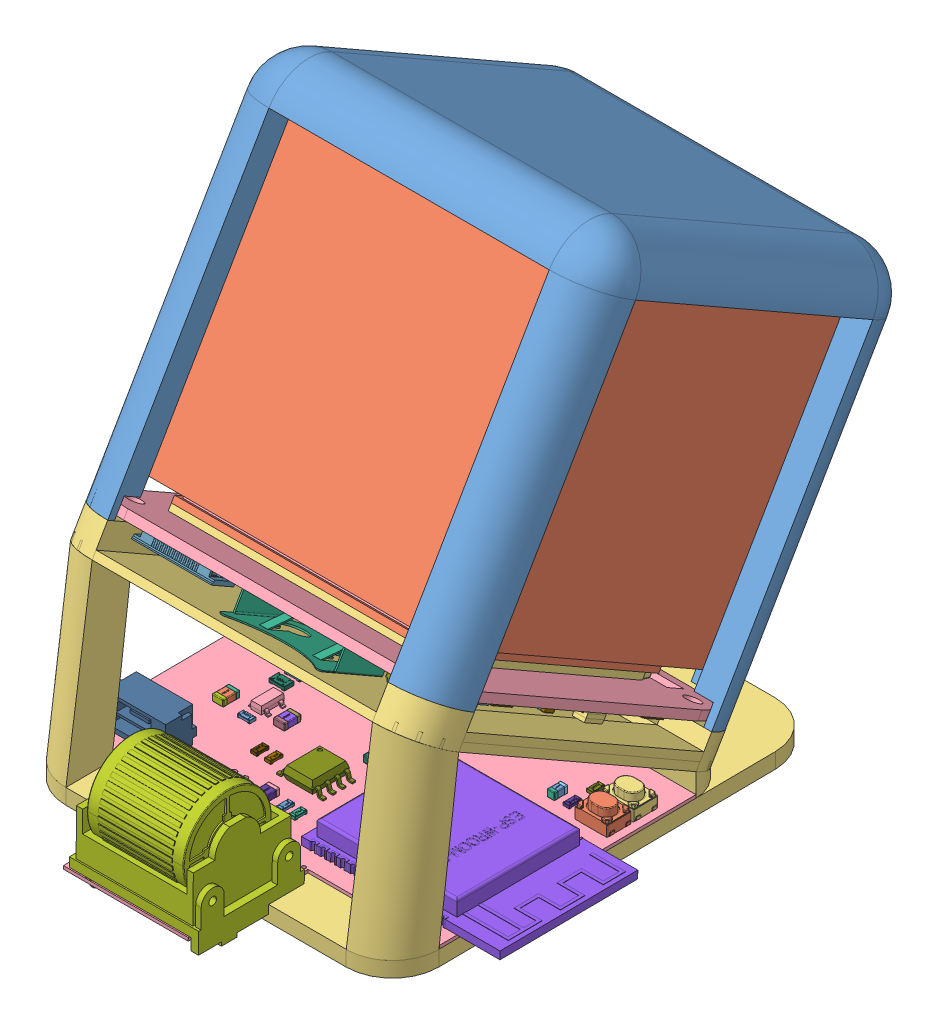
SolidWorks assembly main, configuration 默认. Lengths in mm. (continued)
Components (placement in the parent): (continued)
- PCB_deskclok_ext_2021-02-23-1: PCB_deskclok_ext_2021-02-23 [默认] at (-67.7963 -6.5111 77.6298) x (0.999924 -0.008726 -0.008727) z (0.008727 0.999962 0) size (54.77 48.92 16.75)
  - PCB_deskclok_ext_2021-02-23(2)^PCB_deskclok_ext_2021-02-23-1: PCB_deskclok_ext_2021-02-23(2)^PCB_deskclok_ext_2021-02-23 [默认] at origin size (54.77 48.92 16.75) (virtual)
    - Board^PCB_deskclok_ext_2021-02-23(2)_PCB_deskclok_ext_2021-02-23-1: Board^PCB_deskclok_ext_2021-02-23(2)_PCB_deskclok_ext_2021-02-23 [默认] at origin size (48 48.92 0.41) (virtual)
      - Open CASCADE STEP translator 6.8 2.1.1^Board_PCB_deskclok_ext_2021-02-23(2)_PCB_deskclok_ext_2021-02-23-1: Open CASCADE STEP translator 6.8 2.1.1^Board_PCB_deskclok_ext_2021-02-23(2)_PCB_deskclok_ext_2021-02-23 [默认] at (0 0 -0.4115) size (48 48.92 0.41) (virtual)
        - Open CASCADE STEP translator 6.8 2.1.1.1^Open CASCADE STEP translator 6.8 2.1.1_Board_PCB_deskclok_ext_2021-02-23(2)_PCB_deskclok_ext_2021-02-23-1: Open CASCADE STEP translator 6.8 2.1.1.1^Open CASCADE STEP translator 6.8 2.1.1_Board_PCB_deskclok_ext_2021-02-23(2)_PCB_deskclok_ext_2021-02-23 [默认] at origin size (48 48.92 0.41) (virtual)
    - LED6^PCB_deskclok_ext_2021-02-23(2)_PCB_deskclok_ext_2021-02-23-1: LED6^PCB_deskclok_ext_2021-02-23(2)_PCB_deskclok_ext_2021-02-23 [默认] at origin size (2.13 1.25 1.24) (virtual)
      - everlight-17-21-0805LED-GREEN^LED6_PCB_deskclok_ext_2021-02-23(2)_PCB_deskclok_ext_2021-02-23-1: everlight-17-21-0805LED-GREEN^LED6_PCB_deskclok_ext_2021-02-23(2)_PCB_deskclok_ext_2021-02-23 [默认] at (47.3416 90.4196 0.3048) x (1 0 0) z (0 -1 0) size (2.13 1.24 1.25) (virtual)
    - R9^PCB_deskclok_ext_2021-02-23(2)_PCB_deskclok_ext_2021-02-23-1: R9^PCB_deskclok_ext_2021-02-23(2)_PCB_deskclok_ext_2021-02-23 [默认] at origin size (0.8 1.6 0.42) (virtual)
      - User_Library-Res-0603^R9_PCB_deskclok_ext_2021-02-23(2)_PCB_deskclok_ext_2021-02-23-1: User_Library-Res-0603^R9_PCB_deskclok_ext_2021-02-23(2)_PCB_deskclok_ext_2021-02-23 [默认] at (69.3811 64.135 0) x (0 -1 0) z (-1 0 0) size (1.6 0.42 0.8) (virtual)
    - C6^PCB_deskclok_ext_2021-02-23(2)_PCB_deskclok_ext_2021-02-23-1: C6^PCB_deskclok_ext_2021-02-23(2)_PCB_deskclok_ext_2021-02-23 [默认] at origin size (1.45 2.2 0.88) (virtual)
      - c0805c101k5gactu^C6_PCB_deskclok_ext_2021-02-23(2)_PCB_deskclok_ext_2021-02-23-1: c0805c101k5gactu^C6_PCB_deskclok_ext_2021-02-23(2)_PCB_deskclok_ext_2021-02-23 [默认] at (28.223 186.145 -10.6426) x (0 1 0) z (1 0 0) size (2.2 0.88 1.45) (virtual)
        - Open CASCADE STEP translator 6.8 2.4.1.1^c0805c101k5gactu_C6_PCB_deskclok_ext_2021-02-23(2)_PCB_deskclok_ext_2021-02-23-1: Open CASCADE STEP translator 6.8 2.4.1.1^c0805c101k5gactu_C6_PCB_deskclok_ext_2021-02-23(2)_PCB_deskclok_ext_2021-02-23 [默认] at origin size (2 0.86 1.43) (virtual)
        - Open CASCADE STEP translator 6.8 2.4.1.2^c0805c101k5gactu_C6_PCB_deskclok_ext_2021-02-23(2)_PCB_deskclok_ext_2021-02-23-1: Open CASCADE STEP translator 6.8 2.4.1.2^c0805c101k5gactu_C6_PCB_deskclok_ext_2021-02-23(2)_PCB_deskclok_ext_2021-02-23 [默认] at origin size (0.34 0 0.18) (virtual)
        - Open CASCADE STEP translator 6.8 2.4.1.3^c0805c101k5gactu_C6_PCB_deskclok_ext_2021-02-23(2)_PCB_deskclok_ext_2021-02-23-1: Open CASCADE STEP translator 6.8 2.4.1.3^c0805c101k5gactu_C6_PCB_deskclok_ext_2021-02-23(2)_PCB_deskclok_ext_2021-02-23 [默认] at origin size (0.41 0 0.18) (virtual)
        - Open CASCADE STEP translator 6.8 2.4.1.4^c0805c101k5gactu_C6_PCB_deskclok_ext_2021-02-23(2)_PCB_deskclok_ext_2021-02-23-1: Open CASCADE STEP translator 6.8 2.4.1.4^c0805c101k5gactu_C6_PCB_deskclok_ext_2021-02-23(2)_PCB_deskclok_ext_2021-02-23 [默认] at origin size (0.21 0 0.18) (virtual)
        - Open CASCADE STEP translator 6.8 2.4.1.5^c0805c101k5gactu_C6_PCB_deskclok_ext_2021-02-23(2)_PCB_deskclok_ext_2021-02-23-1: Open CASCADE STEP translator 6.8 2.4.1.5^c0805c101k5gactu_C6_PCB_deskclok_ext_2021-02-23(2)_PCB_deskclok_ext_2021-02-23 [默认] at origin size (0.5 0.88 1.45) (virtual)
        - Open CASCADE STEP translator 6.8 2.4.1.6^c0805c101k5gactu_C6_PCB_deskclok_ext_2021-02-23(2)_PCB_deskclok_ext_2021-02-23-1: Open CASCADE STEP translator 6.8 2.4.1.6^c0805c101k5gactu_C6_PCB_deskclok_ext_2021-02-23(2)_PCB_deskclok_ext_2021-02-23 [默认] at origin size (0.5 0.88 1.45) (virtual)
    - C9^PCB_deskclok_ext_2021-02-23(2)_PCB_deskclok_ext_2021-02-23-1: C9^PCB_deskclok_ext_2021-02-23(2)_PCB_deskclok_ext_2021-02-23 [默认] at origin size (1.45 2.2 0.88) (virtual)
      - c0805c101k5gactu^C9_PCB_deskclok_ext_2021-02-23(2)_PCB_deskclok_ext_2021-02-23-1: c0805c101k5gactu^C9_PCB_deskclok_ext_2021-02-23(2)_PCB_deskclok_ext_2021-02-23 [默认] at (117.778 -11.52 -10.6426) x (0 -1 0) z (-1 0 0) size (2.2 0.88 1.45) (virtual)
        - Open CASCADE STEP translator 6.8 2.4.1.1^c0805c101k5gactu_C9_PCB_deskclok_ext_2021-02-23(2)_PCB_deskclok_ext_2021-02-23-1: Open CASCADE STEP translator 6.8 2.4.1.1^c0805c101k5gactu_C9_PCB_deskclok_ext_2021-02-23(2)_PCB_deskclok_ext_2021-02-23 [默认] at origin size (2 0.86 1.43) (virtual)
        - Open CASCADE STEP translator 6.8 2.4.1.2^c0805c101k5gactu_C9_PCB_deskclok_ext_2021-02-23(2)_PCB_deskclok_ext_2021-02-23-1: Open CASCADE STEP translator 6.8 2.4.1.2^c0805c101k5gactu_C9_PCB_deskclok_ext_2021-02-23(2)_PCB_deskclok_ext_2021-02-23 [默认] at origin size (0.34 0 0.18) (virtual)
        - Open CASCADE STEP translator 6.8 2.4.1.3^c0805c101k5gactu_C9_PCB_deskclok_ext_2021-02-23(2)_PCB_deskclok_ext_2021-02-23-1: Open CASCADE STEP translator 6.8 2.4.1.3^c0805c101k5gactu_C9_PCB_deskclok_ext_2021-02-23(2)_PCB_deskclok_ext_2021-02-23 [默认] at origin size (0.41 0 0.18) (virtual)
        - Open CASCADE STEP translator 6.8 2.4.1.4^c0805c101k5gactu_C9_PCB_deskclok_ext_2021-02-23(2)_PCB_deskclok_ext_2021-02-23-1: Open CASCADE STEP translator 6.8 2.4.1.4^c0805c101k5gactu_C9_PCB_deskclok_ext_2021-02-23(2)_PCB_deskclok_ext_2021-02-23 [默认] at origin size (0.21 0 0.18) (virtual)
        - Open CASCADE STEP translator 6.8 2.4.1.5^c0805c101k5gactu_C9_PCB_deskclok_ext_2021-02-23(2)_PCB_deskclok_ext_2021-02-23-1: Open CASCADE STEP translator 6.8 2.4.1.5^c0805c101k5gactu_C9_PCB_deskclok_ext_2021-02-23(2)_PCB_deskclok_ext_2021-02-23 [默认] at origin size (0.5 0.88 1.45) (virtual)
        - Open CASCADE STEP translator 6.8 2.4.1.6^c0805c101k5gactu_C9_PCB_deskclok_ext_2021-02-23(2)_PCB_deskclok_ext_2021-02-23-1: Open CASCADE STEP translator 6.8 2.4.1.6^c0805c101k5gactu_C9_PCB_deskclok_ext_2021-02-23(2)_PCB_deskclok_ext_2021-02-23 [默认] at origin size (0.5 0.88 1.45) (virtual)
    - R1^PCB_deskclok_ext_2021-02-23(2)_PCB_deskclok_ext_2021-02-23-1: R1^PCB_deskclok_ext_2021-02-23(2)_PCB_deskclok_ext_2021-02-23 [默认] at origin size (1.6 0.8 0.42) (virtual)
      - User_Library-Res-0603^R1_PCB_deskclok_ext_2021-02-23(2)_PCB_deskclok_ext_2021-02-23-1: User_Library-Res-0603^R1_PCB_deskclok_ext_2021-02-23(2)_PCB_deskclok_ext_2021-02-23 [默认] at (55.411 71.6281 0) x (1 0 0) z (0 -1 0) size (1.6 0.42 0.8) (virtual)
    - C1^PCB_deskclok_ext_2021-02-23(2)_PCB_deskclok_ext_2021-02-23-1: C1^PCB_deskclok_ext_2021-02-23(2)_PCB_deskclok_ext_2021-02-23 [默认] at origin size (1.45 2.2 0.88) (virtual)
      - c0805c101k5gactu^C1_PCB_deskclok_ext_2021-02-23(2)_PCB_deskclok_ext_2021-02-23-1: c0805c101k5gactu^C1_PCB_deskclok_ext_2021-02-23(2)_PCB_deskclok_ext_2021-02-23 [默认] at (8.411 169.254 -10.6426) x (0 1 0) z (1 0 0) size (2.2 0.88 1.45) (virtual)
        - Open CASCADE STEP translator 6.8 2.4.1.1^c0805c101k5gactu_C1_PCB_deskclok_ext_2021-02-23(2)_PCB_deskclok_ext_2021-02-23-1: Open CASCADE STEP translator 6.8 2.4.1.1^c0805c101k5gactu_C1_PCB_deskclok_ext_2021-02-23(2)_PCB_deskclok_ext_2021-02-23 [默认] at origin size (2 0.86 1.43) (virtual)
        - Open CASCADE STEP translator 6.8 2.4.1.2^c0805c101k5gactu_C1_PCB_deskclok_ext_2021-02-23(2)_PCB_deskclok_ext_2021-02-23-1: Open CASCADE STEP translator 6.8 2.4.1.2^c0805c101k5gactu_C1_PCB_deskclok_ext_2021-02-23(2)_PCB_deskclok_ext_2021-02-23 [默认] at origin size (0.34 0 0.18) (virtual)
        - Open CASCADE STEP translator 6.8 2.4.1.3^c0805c101k5gactu_C1_PCB_deskclok_ext_2021-02-23(2)_PCB_deskclok_ext_2021-02-23-1: Open CASCADE STEP translator 6.8 2.4.1.3^c0805c101k5gactu_C1_PCB_deskclok_ext_2021-02-23(2)_PCB_deskclok_ext_2021-02-23 [默认] at origin size (0.41 0 0.18) (virtual)
        - Open CASCADE STEP translator 6.8 2.4.1.4^c0805c101k5gactu_C1_PCB_deskclok_ext_2021-02-23(2)_PCB_deskclok_ext_2021-02-23-1: Open CASCADE STEP translator 6.8 2.4.1.4^c0805c101k5gactu_C1_PCB_deskclok_ext_2021-02-23(2)_PCB_deskclok_ext_2021-02-23 [默认] at origin size (0.21 0 0.18) (virtual)
        - Open CASCADE STEP translator 6.8 2.4.1.5^c0805c101k5gactu_C1_PCB_deskclok_ext_2021-02-23(2)_PCB_deskclok_ext_2021-02-23-1: Open CASCADE STEP translator 6.8 2.4.1.5^c0805c101k5gactu_C1_PCB_deskclok_ext_2021-02-23(2)_PCB_deskclok_ext_2021-02-23 [默认] at origin size (0.5 0.88 1.45) (virtual)
        - Open CASCADE STEP translator 6.8 2.4.1.6^c0805c101k5gactu_C1_PCB_deskclok_ext_2021-02-23(2)_PCB_deskclok_ext_2021-02-23-1: Open CASCADE STEP translator 6.8 2.4.1.6^c0805c101k5gactu_C1_PCB_deskclok_ext_2021-02-23(2)_PCB_deskclok_ext_2021-02-23 [默认] at origin size (0.5 0.88 1.45) (virtual)
    - C2^PCB_deskclok_ext_2021-02-23(2)_PCB_deskclok_ext_2021-02-23-1: C2^PCB_deskclok_ext_2021-02-23(2)_PCB_deskclok_ext_2021-02-23 [默认] at origin size (1.45 2.2 0.88) (virtual)
      - c0805c101k5gactu^C2_PCB_deskclok_ext_2021-02-23(2)_PCB_deskclok_ext_2021-02-23-1: c0805c101k5gactu^C2_PCB_deskclok_ext_2021-02-23(2)_PCB_deskclok_ext_2021-02-23 [默认] at (15.015 170.524 -10.6426) x (0 1 0) z (1 0 0) size (2.2 0.88 1.45) (virtual)
        - Open CASCADE STEP translator 6.8 2.4.1.1^c0805c101k5gactu_C2_PCB_deskclok_ext_2021-02-23(2)_PCB_deskclok_ext_2021-02-23-1: Open CASCADE STEP translator 6.8 2.4.1.1^c0805c101k5gactu_C2_PCB_deskclok_ext_2021-02-23(2)_PCB_deskclok_ext_2021-02-23 [默认] at origin size (2 0.86 1.43) (virtual)
        - Open CASCADE STEP translator 6.8 2.4.1.2^c0805c101k5gactu_C2_PCB_deskclok_ext_2021-02-23(2)_PCB_deskclok_ext_2021-02-23-1: Open CASCADE STEP translator 6.8 2.4.1.2^c0805c101k5gactu_C2_PCB_deskclok_ext_2021-02-23(2)_PCB_deskclok_ext_2021-02-23 [默认] at origin size (0.34 0 0.18) (virtual)
        - Open CASCADE STEP translator 6.8 2.4.1.3^c0805c101k5gactu_C2_PCB_deskclok_ext_2021-02-23(2)_PCB_deskclok_ext_2021-02-23-1: Open CASCADE STEP translator 6.8 2.4.1.3^c0805c101k5gactu_C2_PCB_deskclok_ext_2021-02-23(2)_PCB_deskclok_ext_2021-02-23 [默认] at origin size (0.41 0 0.18) (virtual)
        - Open CASCADE STEP translator 6.8 2.4.1.4^c0805c101k5gactu_C2_PCB_deskclok_ext_2021-02-23(2)_PCB_deskclok_ext_2021-02-23-1: Open CASCADE STEP translator 6.8 2.4.1.4^c0805c101k5gactu_C2_PCB_deskclok_ext_2021-02-23(2)_PCB_deskclok_ext_2021-02-23 [默认] at origin size (0.21 0 0.18) (virtual)
        - Open CASCADE STEP translator 6.8 2.4.1.5^c0805c101k5gactu_C2_PCB_deskclok_ext_2021-02-23(2)_PCB_deskclok_ext_2021-02-23-1: Open CASCADE STEP translator 6.8 2.4.1.5^c0805c101k5gactu_C2_PCB_deskclok_ext_2021-02-23(2)_PCB_deskclok_ext_2021-02-23 [默认] at origin size (0.5 0.88 1.45) (virtual)
        - Open CASCADE STEP translator 6.8 2.4.1.6^c0805c101k5gactu_C2_PCB_deskclok_ext_2021-02-23(2)_PCB_deskclok_ext_2021-02-23-1: Open CASCADE STEP translator 6.8 2.4.1.6^c0805c101k5gactu_C2_PCB_deskclok_ext_2021-02-23(2)_PCB_deskclok_ext_2021-02-23 [默认] at origin size (0.5 0.88 1.45) (virtual)
    - R13^PCB_deskclok_ext_2021-02-23(2)_PCB_deskclok_ext_2021-02-23-1: R13^PCB_deskclok_ext_2021-02-23(2)_PCB_deskclok_ext_2021-02-23 [默认] at origin size (2 1.25 0.53) (virtual)
      - User_Library-Res-0805^R13_PCB_deskclok_ext_2021-02-23(2)_PCB_deskclok_ext_2021-02-23-1: User_Library-Res-0805^R13_PCB_deskclok_ext_2021-02-23(2)_PCB_deskclok_ext_2021-02-23 [默认] at (54.1409 79.4919 0.3048) x (1 0 0) z (0 -1 0) size (2 0.53 1.25) (virtual)
    - R14^PCB_deskclok_ext_2021-02-23(2)_PCB_deskclok_ext_2021-02-23-1: R14^PCB_deskclok_ext_2021-02-23(2)_PCB_deskclok_ext_2021-02-23 [默认] at origin size (2 1.25 0.53) (virtual)
      - User_Library-Res-0805^R14_PCB_deskclok_ext_2021-02-23(2)_PCB_deskclok_ext_2021-02-23-1: User_Library-Res-0805^R14_PCB_deskclok_ext_2021-02-23(2)_PCB_deskclok_ext_2021-02-23 [默认] at (54.141 77.4801 0.3048) x (-1 0 0) z (0 1 0) size (2 0.53 1.25) (virtual)
    - U3^PCB_deskclok_ext_2021-02-23(2)_PCB_deskclok_ext_2021-02-23-1: U3^PCB_deskclok_ext_2021-02-23(2)_PCB_deskclok_ext_2021-02-23 [默认] at origin size (6 4.9 1.7) (virtual)
      - User_Library-so8-3^U3_PCB_deskclok_ext_2021-02-23(2)_PCB_deskclok_ext_2021-02-23-1: User_Library-so8-3^U3_PCB_deskclok_ext_2021-02-23(2)_PCB_deskclok_ext_2021-02-23 [默认] at (66.4601 69.469 0) x (1 0 0) z (0 0 1) size (6 4.9 1.7) (virtual)
    - U9^PCB_deskclok_ext_2021-02-23(2)_PCB_deskclok_ext_2021-02-23-1: U9^PCB_deskclok_ext_2021-02-23(2)_PCB_deskclok_ext_2021-02-23 [默认] at origin size (3 2.5 1.1) (virtual)
      - CircuitWorks-SOT-23-5^U9_PCB_deskclok_ext_2021-02-23(2)_PCB_deskclok_ext_2021-02-23-1: CircuitWorks-SOT-23-5^U9_PCB_deskclok_ext_2021-02-23(2)_PCB_deskclok_ext_2021-02-23 [默认] at (68.536 88.8961 0.5588) x (-1 0 0) z (0 1 0) size (3 1.1 2.5) (virtual)
    - FPC3^PCB_deskclok_ext_2021-02-23(2)_PCB_deskclok_ext_2021-02-23-1: FPC3^PCB_deskclok_ext_2021-02-23(2)_PCB_deskclok_ext_2021-02-23 [默认] at origin size (12.1 6.6 2) (virtual)
      - 52746-1290_RGB10066329^FPC3_PCB_deskclok_ext_2021-02-23(2)_PCB_deskclok_ext_2021-02-23-1: 52746-1290_RGB10066329^FPC3_PCB_deskclok_ext_2021-02-23(2)_PCB_deskclok_ext_2021-02-23 [默认] at (58.4591 88.7731 0) x (1 0 0) z (0 -1 0) size (12.1 2 6.6) (virtual)
    - C35^PCB_deskclok_ext_2021-02-23(2)_PCB_deskclok_ext_2021-02-23-1: C35^PCB_deskclok_ext_2021-02-23(2)_PCB_deskclok_ext_2021-02-23 [默认] at origin size (0.95 1.77 0.95) (virtual)
      - c0603x104k3ractu^C35_PCB_deskclok_ext_2021-02-23(2)_PCB_deskclok_ext_2021-02-23-1: c0603x104k3ractu^C35_PCB_deskclok_ext_2021-02-23(2)_PCB_deskclok_ext_2021-02-23 [默认] at (40.1705 179.789 -10.6426) x (0 1 0) z (1 0 0) size (1.77 0.95 0.95) (virtual)
        - Open CASCADE STEP translator 6.8 2.14.1.1^c0603x104k3ractu_C35_PCB_deskclok_ext_2021-02-23(2)_PCB_deskclok_ext_2021-02-23-1: Open CASCADE STEP translator 6.8 2.14.1.1^c0603x104k3ractu_C35_PCB_deskclok_ext_2021-02-23(2)_PCB_deskclok_ext_2021-02-23 [默认] at origin size (1.57 0.93 0.93) (virtual)
        - Open CASCADE STEP translator 6.8 2.14.1.2^c0603x104k3ractu_C35_PCB_deskclok_ext_2021-02-23(2)_PCB_deskclok_ext_2021-02-23-1: Open CASCADE STEP translator 6.8 2.14.1.2^c0603x104k3ractu_C35_PCB_deskclok_ext_2021-02-23(2)_PCB_deskclok_ext_2021-02-23 [默认] at origin size (0.24 0 0.13) (virtual)
        - Open CASCADE STEP translator 6.8 2.14.1.3^c0603x104k3ractu_C35_PCB_deskclok_ext_2021-02-23(2)_PCB_deskclok_ext_2021-02-23-1: Open CASCADE STEP translator 6.8 2.14.1.3^c0603x104k3ractu_C35_PCB_deskclok_ext_2021-02-23(2)_PCB_deskclok_ext_2021-02-23 [默认] at origin size (0.29 0 0.13) (virtual)
        - Open CASCADE STEP translator 6.8 2.14.1.4^c0603x104k3ractu_C35_PCB_deskclok_ext_2021-02-23(2)_PCB_deskclok_ext_2021-02-23-1: Open CASCADE STEP translator 6.8 2.14.1.4^c0603x104k3ractu_C35_PCB_deskclok_ext_2021-02-23(2)_PCB_deskclok_ext_2021-02-23 [默认] at origin size (0.15 0 0.13) (virtual)
        - Open CASCADE STEP translator 6.8 2.14.1.5^c0603x104k3ractu_C35_PCB_deskclok_ext_2021-02-23(2)_PCB_deskclok_ext_2021-02-23-1: Open CASCADE STEP translator 6.8 2.14.1.5^c0603x104k3ractu_C35_PCB_deskclok_ext_2021-02-23(2)_PCB_deskclok_ext_2021-02-23 [默认] at origin size (0.45 0.95 0.95) (virtual)
        - Open CASCADE STEP translator 6.8 2.14.1.6^c0603x104k3ractu_C35_PCB_deskclok_ext_2021-02-23(2)_PCB_deskclok_ext_2021-02-23-1: Open CASCADE STEP translator 6.8 2.14.1.6^c0603x104k3ractu_C35_PCB_deskclok_ext_2021-02-23(2)_PCB_deskclok_ext_2021-02-23 [默认] at origin size (0.45 0.95 0.95) (virtual)
    - D1^PCB_deskclok_ext_2021-02-23(2)_PCB_deskclok_ext_2021-02-23-1: D1^PCB_deskclok_ext_2021-02-23(2)_PCB_deskclok_ext_2021-02-23 [默认] at origin size (2.6 1.35 1.1) (virtual)
      - User_Library-SOD323-1^D1_PCB_deskclok_ext_2021-02-23(2)_PCB_deskclok_ext_2021-02-23-1: User_Library-SOD323-1^D1_PCB_deskclok_ext_2021-02-23(2)_PCB_deskclok_ext_2021-02-23 [默认] at (50.9659 85.0899 0) x (-1 0 0) z (0 0 1) size (2.6 1.35 1.1) (virtual)
    - R4^PCB_deskclok_ext_2021-02-23(2)_PCB_deskclok_ext_2021-02-23-1: R4^PCB_deskclok_ext_2021-02-23(2)_PCB_deskclok_ext_2021-02-23 [默认] at origin size (1.6 0.8 0.42) (virtual)
      - User_Library-Res-0603^R4_PCB_deskclok_ext_2021-02-23(2)_PCB_deskclok_ext_2021-02-23-1: User_Library-Res-0603^R4_PCB_deskclok_ext_2021-02-23(2)_PCB_deskclok_ext_2021-02-23 [默认] at (66.2059 85.7249 0) x (-1 0 0) z (0 1 0) size (1.6 0.42 0.8) (virtual)
    - R8^PCB_deskclok_ext_2021-02-23(2)_PCB_deskclok_ext_2021-02-23-1: R8^PCB_deskclok_ext_2021-02-23(2)_PCB_deskclok_ext_2021-02-23 [默认] at origin size (0.8 1.6 0.42) (virtual)
      - User_Library-Res-0603^R8_PCB_deskclok_ext_2021-02-23(2)_PCB_deskclok_ext_2021-02-23-1: User_Library-Res-0603^R8_PCB_deskclok_ext_2021-02-23(2)_PCB_deskclok_ext_2021-02-23 [默认] at (61.6341 68.834 0) x (0 -1 0) z (-1 0 0) size (1.6 0.42 0.8) (virtual)
    - C4^PCB_deskclok_ext_2021-02-23(2)_PCB_deskclok_ext_2021-02-23-1: C4^PCB_deskclok_ext_2021-02-23(2)_PCB_deskclok_ext_2021-02-23 [默认] at origin size (1.45 2.2 0.88) (virtual)
      - c0805c101k5gactu^C4_PCB_deskclok_ext_2021-02-23(2)_PCB_deskclok_ext_2021-02-23-1: c0805c101k5gactu^C4_PCB_deskclok_ext_2021-02-23(2)_PCB_deskclok_ext_2021-02-23 [默认] at (24.921 172.175 -10.6426) x (0 1 0) z (1 0 0) size (2.2 0.88 1.45) (virtual)
        - Open CASCADE STEP translator 6.8 2.4.1.1^c0805c101k5gactu_C4_PCB_deskclok_ext_2021-02-23(2)_PCB_deskclok_ext_2021-02-23-1: Open CASCADE STEP translator 6.8 2.4.1.1^c0805c101k5gactu_C4_PCB_deskclok_ext_2021-02-23(2)_PCB_deskclok_ext_2021-02-23 [默认] at origin size (2 0.86 1.43) (virtual)
        - Open CASCADE STEP translator 6.8 2.4.1.2^c0805c101k5gactu_C4_PCB_deskclok_ext_2021-02-23(2)_PCB_deskclok_ext_2021-02-23-1: Open CASCADE STEP translator 6.8 2.4.1.2^c0805c101k5gactu_C4_PCB_deskclok_ext_2021-02-23(2)_PCB_deskclok_ext_2021-02-23 [默认] at origin size (0.34 0 0.18) (virtual)
        - Open CASCADE STEP translator 6.8 2.4.1.3^c0805c101k5gactu_C4_PCB_deskclok_ext_2021-02-23(2)_PCB_deskclok_ext_2021-02-23-1: Open CASCADE STEP translator 6.8 2.4.1.3^c0805c101k5gactu_C4_PCB_deskclok_ext_2021-02-23(2)_PCB_deskclok_ext_2021-02-23 [默认] at origin size (0.41 0 0.18) (virtual)
        - Open CASCADE STEP translator 6.8 2.4.1.4^c0805c101k5gactu_C4_PCB_deskclok_ext_2021-02-23(2)_PCB_deskclok_ext_2021-02-23-1: Open CASCADE STEP translator 6.8 2.4.1.4^c0805c101k5gactu_C4_PCB_deskclok_ext_2021-02-23(2)_PCB_deskclok_ext_2021-02-23 [默认] at origin size (0.21 0 0.18) (virtual)
        - Open CASCADE STEP translator 6.8 2.4.1.5^c0805c101k5gactu_C4_PCB_deskclok_ext_2021-02-23(2)_PCB_deskclok_ext_2021-02-23-1: Open CASCADE STEP translator 6.8 2.4.1.5^c0805c101k5gactu_C4_PCB_deskclok_ext_2021-02-23(2)_PCB_deskclok_ext_2021-02-23 [默认] at origin size (0.5 0.88 1.45) (virtual)
        - Open CASCADE STEP translator 6.8 2.4.1.6^c0805c101k5gactu_C4_PCB_deskclok_ext_2021-02-23(2)_PCB_deskclok_ext_2021-02-23-1: Open CASCADE STEP translator 6.8 2.4.1.6^c0805c101k5gactu_C4_PCB_deskclok_ext_2021-02-23(2)_PCB_deskclok_ext_2021-02-23 [默认] at origin size (0.5 0.88 1.45) (virtual)
    - R7^PCB_deskclok_ext_2021-02-23(2)_PCB_deskclok_ext_2021-02-23-1: R7^PCB_deskclok_ext_2021-02-23(2)_PCB_deskclok_ext_2021-02-23 [默认] at origin size (0.8 1.6 0.42) (virtual)
      - User_Library-Res-0603^R7_PCB_deskclok_ext_2021-02-23(2)_PCB_deskclok_ext_2021-02-23-1: User_Library-Res-0603^R7_PCB_deskclok_ext_2021-02-23(2)_PCB_deskclok_ext_2021-02-23 [默认] at (85.8909 86.233 0) x (0 1 0) z (1 0 0) size (1.6 0.42 0.8) (virtual)
    - R6^PCB_deskclok_ext_2021-02-23(2)_PCB_deskclok_ext_2021-02-23-1: R6^PCB_deskclok_ext_2021-02-23(2)_PCB_deskclok_ext_2021-02-23 [默认] at origin size (0.8 1.6 0.42) (virtual)
      - User_Library-Res-0603^R6_PCB_deskclok_ext_2021-02-23(2)_PCB_deskclok_ext_2021-02-23-1: User_Library-Res-0603^R6_PCB_deskclok_ext_2021-02-23(2)_PCB_deskclok_ext_2021-02-23 [默认] at (85.8911 83.185 0) x (0 -1 0) z (-1 0 0) size (1.6 0.42 0.8) (virtual)
    - R3^PCB_deskclok_ext_2021-02-23(2)_PCB_deskclok_ext_2021-02-23-1: R3^PCB_deskclok_ext_2021-02-23(2)_PCB_deskclok_ext_2021-02-23 [默认] at origin size (0.8 1.6 0.42) (virtual)
      - User_Library-Res-0603^R3_PCB_deskclok_ext_2021-02-23(2)_PCB_deskclok_ext_2021-02-23-1: User_Library-Res-0603^R3_PCB_deskclok_ext_2021-02-23(2)_PCB_deskclok_ext_2021-02-23 [默认] at (59.8559 68.834 0) x (0 1 0) z (1 0 0) size (1.6 0.42 0.8) (virtual)
    - R2^PCB_deskclok_ext_2021-02-23(2)_PCB_deskclok_ext_2021-02-23-1: R2^PCB_deskclok_ext_2021-02-23(2)_PCB_deskclok_ext_2021-02-23 [默认] at origin size (0.8 1.6 0.42) (virtual)
      - User_Library-Res-0603^R2_PCB_deskclok_ext_2021-02-23(2)_PCB_deskclok_ext_2021-02-23-1: User_Library-Res-0603^R2_PCB_deskclok_ext_2021-02-23(2)_PCB_deskclok_ext_2021-02-23 [默认] at (67.7301 64.135 0) x (0 -1 0) z (-1 0 0) size (1.6 0.42 0.8) (virtual)
    - SW1^PCB_deskclok_ext_2021-02-23(2)_PCB_deskclok_ext_2021-02-23-1: SW1^PCB_deskclok_ext_2021-02-23(2)_PCB_deskclok_ext_2021-02-23 [默认] at origin size (4.6 3.2 2.5) (virtual)
      - skrpace010_RGB10066329^SW1_PCB_deskclok_ext_2021-02-23(2)_PCB_deskclok_ext_2021-02-23-1: skrpace010_RGB10066329^SW1_PCB_deskclok_ext_2021-02-23(2)_PCB_deskclok_ext_2021-02-23 [默认] at (89.8279 83.185 0) x (-1 0 0) z (0 1 0) size (4.6 2.5 3.2) (virtual)
    - SW2^PCB_deskclok_ext_2021-02-23(2)_PCB_deskclok_ext_2021-02-23-1: SW2^PCB_deskclok_ext_2021-02-23(2)_PCB_deskclok_ext_2021-02-23 [默认] at origin size (4.6 3.2 2.5) (virtual)
      - skrpace010_RGB10066329^SW2_PCB_deskclok_ext_2021-02-23(2)_PCB_deskclok_ext_2021-02-23-1: skrpace010_RGB10066329^SW2_PCB_deskclok_ext_2021-02-23(2)_PCB_deskclok_ext_2021-02-23 [默认] at (89.8281 86.614 0) x (1 0 0) z (0 -1 0) size (4.6 2.5 3.2) (virtual)
    - U1^PCB_deskclok_ext_2021-02-23(2)_PCB_deskclok_ext_2021-02-23-1: U1^PCB_deskclok_ext_2021-02-23(2)_PCB_deskclok_ext_2021-02-23 [默认] at origin size (2.5 3 1.1) (virtual)
      - CircuitWorks-SOT-23-5^U1_PCB_deskclok_ext_2021-02-23(2)_PCB_deskclok_ext_2021-02-23-1: CircuitWorks-SOT-23-5^U1_PCB_deskclok_ext_2021-02-23(2)_PCB_deskclok_ext_2021-02-23 [默认] at (55.4148 74.339 0.5588) x (0 -1 0) z (-1 0 0) size (3 1.1 2.5) (virtual)
    - C7^PCB_deskclok_ext_2021-02-23(2)_PCB_deskclok_ext_2021-02-23-1: C7^PCB_deskclok_ext_2021-02-23(2)_PCB_deskclok_ext_2021-02-23 [默认] at origin size (1.45 2.2 0.88) (virtual)
      - c0805c101k5gactu^C7_PCB_deskclok_ext_2021-02-23(2)_PCB_deskclok_ext_2021-02-23-1: c0805c101k5gactu^C7_PCB_deskclok_ext_2021-02-23(2)_PCB_deskclok_ext_2021-02-23 [默认] at (117.778 -7.583 -10.6426) x (0 -1 0) z (-1 0 0) size (2.2 0.88 1.45) (virtual)
        - Open CASCADE STEP translator 6.8 2.4.1.1^c0805c101k5gactu_C7_PCB_deskclok_ext_2021-02-23(2)_PCB_deskclok_ext_2021-02-23-1: Open CASCADE STEP translator 6.8 2.4.1.1^c0805c101k5gactu_C7_PCB_deskclok_ext_2021-02-23(2)_PCB_deskclok_ext_2021-02-23 [默认] at origin size (2 0.86 1.43) (virtual)
        - Open CASCADE STEP translator 6.8 2.4.1.2^c0805c101k5gactu_C7_PCB_deskclok_ext_2021-02-23(2)_PCB_deskclok_ext_2021-02-23-1: Open CASCADE STEP translator 6.8 2.4.1.2^c0805c101k5gactu_C7_PCB_deskclok_ext_2021-02-23(2)_PCB_deskclok_ext_2021-02-23 [默认] at origin size (0.34 0 0.18) (virtual)
        - Open CASCADE STEP translator 6.8 2.4.1.3^c0805c101k5gactu_C7_PCB_deskclok_ext_2021-02-23(2)_PCB_deskclok_ext_2021-02-23-1: Open CASCADE STEP translator 6.8 2.4.1.3^c0805c101k5gactu_C7_PCB_deskclok_ext_2021-02-23(2)_PCB_deskclok_ext_2021-02-23 [默认] at origin size (0.41 0 0.18) (virtual)
        - Open CASCADE STEP translator 6.8 2.4.1.4^c0805c101k5gactu_C7_PCB_deskclok_ext_2021-02-23(2)_PCB_deskclok_ext_2021-02-23-1: Open CASCADE STEP translator 6.8 2.4.1.4^c0805c101k5gactu_C7_PCB_deskclok_ext_2021-02-23(2)_PCB_deskclok_ext_2021-02-23 [默认] at origin size (0.21 0 0.18) (virtual)
        - Open CASCADE STEP translator 6.8 2.4.1.5^c0805c101k5gactu_C7_PCB_deskclok_ext_2021-02-23(2)_PCB_deskclok_ext_2021-02-23-1: Open CASCADE STEP translator 6.8 2.4.1.5^c0805c101k5gactu_C7_PCB_deskclok_ext_2021-02-23(2)_PCB_deskclok_ext_2021-02-23 [默认] at origin size (0.5 0.88 1.45) (virtual)
        - Open CASCADE STEP translator 6.8 2.4.1.6^c0805c101k5gactu_C7_PCB_deskclok_ext_2021-02-23(2)_PCB_deskclok_ext_2021-02-23-1: Open CASCADE STEP translator 6.8 2.4.1.6^c0805c101k5gactu_C7_PCB_deskclok_ext_2021-02-23(2)_PCB_deskclok_ext_2021-02-23 [默认] at origin size (0.5 0.88 1.45) (virtual)
    - C8^PCB_deskclok_ext_2021-02-23(2)_PCB_deskclok_ext_2021-02-23-1: C8^PCB_deskclok_ext_2021-02-23(2)_PCB_deskclok_ext_2021-02-23 [默认] at origin size (1.45 2.2 0.88) (virtual)
      - c0805c101k5gactu^C8_PCB_deskclok_ext_2021-02-23(2)_PCB_deskclok_ext_2021-02-23-1: c0805c101k5gactu^C8_PCB_deskclok_ext_2021-02-23(2)_PCB_deskclok_ext_2021-02-23 [默认] at (115.365 -11.52 -10.6426) x (0 -1 0) z (-1 0 0) size (2.2 0.88 1.45) (virtual)
        - Open CASCADE STEP translator 6.8 2.4.1.1^c0805c101k5gactu_C8_PCB_deskclok_ext_2021-02-23(2)_PCB_deskclok_ext_2021-02-23-1: Open CASCADE STEP translator 6.8 2.4.1.1^c0805c101k5gactu_C8_PCB_deskclok_ext_2021-02-23(2)_PCB_deskclok_ext_2021-02-23 [默认] at origin size (2 0.86 1.43) (virtual)
        - Open CASCADE STEP translator 6.8 2.4.1.2^c0805c101k5gactu_C8_PCB_deskclok_ext_2021-02-23(2)_PCB_deskclok_ext_2021-02-23-1: Open CASCADE STEP translator 6.8 2.4.1.2^c0805c101k5gactu_C8_PCB_deskclok_ext_2021-02-23(2)_PCB_deskclok_ext_2021-02-23 [默认] at origin size (0.34 0 0.18) (virtual)
        - Open CASCADE STEP translator 6.8 2.4.1.3^c0805c101k5gactu_C8_PCB_deskclok_ext_2021-02-23(2)_PCB_deskclok_ext_2021-02-23-1: Open CASCADE STEP translator 6.8 2.4.1.3^c0805c101k5gactu_C8_PCB_deskclok_ext_2021-02-23(2)_PCB_deskclok_ext_2021-02-23 [默认] at origin size (0.41 0 0.18) (virtual)
        - Open CASCADE STEP translator 6.8 2.4.1.4^c0805c101k5gactu_C8_PCB_deskclok_ext_2021-02-23(2)_PCB_deskclok_ext_2021-02-23-1: Open CASCADE STEP translator 6.8 2.4.1.4^c0805c101k5gactu_C8_PCB_deskclok_ext_2021-02-23(2)_PCB_deskclok_ext_2021-02-23 [默认] at origin size (0.21 0 0.18) (virtual)
        - Open CASCADE STEP translator 6.8 2.4.1.5^c0805c101k5gactu_C8_PCB_deskclok_ext_2021-02-23(2)_PCB_deskclok_ext_2021-02-23-1: Open CASCADE STEP translator 6.8 2.4.1.5^c0805c101k5gactu_C8_PCB_deskclok_ext_2021-02-23(2)_PCB_deskclok_ext_2021-02-23 [默认] at origin size (0.5 0.88 1.45) (virtual)
        - Open CASCADE STEP translator 6.8 2.4.1.6^c0805c101k5gactu_C8_PCB_deskclok_ext_2021-02-23(2)_PCB_deskclok_ext_2021-02-23-1: Open CASCADE STEP translator 6.8 2.4.1.6^c0805c101k5gactu_C8_PCB_deskclok_ext_2021-02-23(2)_PCB_deskclok_ext_2021-02-23 [默认] at origin size (0.5 0.88 1.45) (virtual)
    - C3^PCB_deskclok_ext_2021-02-23(2)_PCB_deskclok_ext_2021-02-23-1: C3^PCB_deskclok_ext_2021-02-23(2)_PCB_deskclok_ext_2021-02-23 [默认] at origin size (1.45 2.2 0.88) (virtual)
      - c0805c101k5gactu^C3_PCB_deskclok_ext_2021-02-23(2)_PCB_deskclok_ext_2021-02-23-1: c0805c101k5gactu^C3_PCB_deskclok_ext_2021-02-23(2)_PCB_deskclok_ext_2021-02-23 [默认] at (108.888 -32.729 -10.6426) x (0 -1 0) z (-1 0 0) size (2.2 0.88 1.45) (virtual)
        - Open CASCADE STEP translator 6.8 2.4.1.1^c0805c101k5gactu_C3_PCB_deskclok_ext_2021-02-23(2)_PCB_deskclok_ext_2021-02-23-1: Open CASCADE STEP translator 6.8 2.4.1.1^c0805c101k5gactu_C3_PCB_deskclok_ext_2021-02-23(2)_PCB_deskclok_ext_2021-02-23 [默认] at origin size (2 0.86 1.43) (virtual)
        - Open CASCADE STEP translator 6.8 2.4.1.2^c0805c101k5gactu_C3_PCB_deskclok_ext_2021-02-23(2)_PCB_deskclok_ext_2021-02-23-1: Open CASCADE STEP translator 6.8 2.4.1.2^c0805c101k5gactu_C3_PCB_deskclok_ext_2021-02-23(2)_PCB_deskclok_ext_2021-02-23 [默认] at origin size (0.34 0 0.18) (virtual)
        - Open CASCADE STEP translator 6.8 2.4.1.3^c0805c101k5gactu_C3_PCB_deskclok_ext_2021-02-23(2)_PCB_deskclok_ext_2021-02-23-1: Open CASCADE STEP translator 6.8 2.4.1.3^c0805c101k5gactu_C3_PCB_deskclok_ext_2021-02-23(2)_PCB_deskclok_ext_2021-02-23 [默认] at origin size (0.41 0 0.18) (virtual)
        - Open CASCADE STEP translator 6.8 2.4.1.4^c0805c101k5gactu_C3_PCB_deskclok_ext_2021-02-23(2)_PCB_deskclok_ext_2021-02-23-1: Open CASCADE STEP translator 6.8 2.4.1.4^c0805c101k5gactu_C3_PCB_deskclok_ext_2021-02-23(2)_PCB_deskclok_ext_2021-02-23 [默认] at origin size (0.21 0 0.18) (virtual)
        - Open CASCADE STEP translator 6.8 2.4.1.5^c0805c101k5gactu_C3_PCB_deskclok_ext_2021-02-23(2)_PCB_deskclok_ext_2021-02-23-1: Open CASCADE STEP translator 6.8 2.4.1.5^c0805c101k5gactu_C3_PCB_deskclok_ext_2021-02-23(2)_PCB_deskclok_ext_2021-02-23 [默认] at origin size (0.5 0.88 1.45) (virtual)
        - Open CASCADE STEP translator 6.8 2.4.1.6^c0805c101k5gactu_C3_PCB_deskclok_ext_2021-02-23(2)_PCB_deskclok_ext_2021-02-23-1: Open CASCADE STEP translator 6.8 2.4.1.6^c0805c101k5gactu_C3_PCB_deskclok_ext_2021-02-23(2)_PCB_deskclok_ext_2021-02-23 [默认] at origin size (0.5 0.88 1.45) (virtual)
    - R5^PCB_deskclok_ext_2021-02-23(2)_PCB_deskclok_ext_2021-02-23-1: R5^PCB_deskclok_ext_2021-02-23(2)_PCB_deskclok_ext_2021-02-23 [默认] at origin size (0.8 1.6 0.42) (virtual)
      - User_Library-Res-0603^R5_PCB_deskclok_ext_2021-02-23(2)_PCB_deskclok_ext_2021-02-23-1: User_Library-Res-0603^R5_PCB_deskclok_ext_2021-02-23(2)_PCB_deskclok_ext_2021-02-23 [默认] at (69.3811 83.312 0) x (0 -1 0) z (-1 0 0) size (1.6 0.42 0.8) (virtual)
    - SW3^PCB_deskclok_ext_2021-02-23(2)_PCB_deskclok_ext_2021-02-23-1: SW3^PCB_deskclok_ext_2021-02-23(2)_PCB_deskclok_ext_2021-02-23 [默认] at origin size (5 7.7 1.9) (virtual)
      - User_Library-MSS3_slide_switch_v2^SW3_PCB_deskclok_ext_2021-02-23(2)_PCB_deskclok_ext_2021-02-23-1: User_Library-MSS3_slide_switch_v2^SW3_PCB_deskclok_ext_2021-02-23(2)_PCB_deskclok_ext_2021-02-23 [默认] at (46.3941 83.6929 0) x (0 1 0) z (0 0 1) size (7.7 5 1.9) (virtual)
    - U5^PCB_deskclok_ext_2021-02-23(2)_PCB_deskclok_ext_2021-02-23-1: U5^PCB_deskclok_ext_2021-02-23(2)_PCB_deskclok_ext_2021-02-23 [默认] at origin size (16.6 13.85 16.75) (virtual)
      - Encoder^U5_PCB_deskclok_ext_2021-02-23(2)_PCB_deskclok_ext_2021-02-23-1: Encoder^U5_PCB_deskclok_ext_2021-02-23(2)_PCB_deskclok_ext_2021-02-23 [默认] at (76.9191 43.4839 0) x (0 1 0) z (1 0 0) size (13.85 16.75 16.6) (virtual)
    - U2^PCB_deskclok_ext_2021-02-23(2)_PCB_deskclok_ext_2021-02-23-1: U2^PCB_deskclok_ext_2021-02-23(2)_PCB_deskclok_ext_2021-02-23 [默认] at origin size (25.54 18.07 3.04) (virtual)
      - User_Library-esp-wroom-32^U2_PCB_deskclok_ext_2021-02-23(2)_PCB_deskclok_ext_2021-02-23-1: User_Library-esp-wroom-32^U2_PCB_deskclok_ext_2021-02-23(2)_PCB_deskclok_ext_2021-02-23 [默认] at (72.907 78.995 0) x (0 -1 0) z (-1 0 0) size (18.07 3.04 25.54) (virtual)
    - Q2^PCB_deskclok_ext_2021-02-23(2)_PCB_deskclok_ext_2021-02-23-1: Q2^PCB_deskclok_ext_2021-02-23(2)_PCB_deskclok_ext_2021-02-23 [默认] at origin size (2.5 3 1.1) (virtual)
      - CircuitWorks-SOT-23^Q2_PCB_deskclok_ext_2021-02-23(2)_PCB_deskclok_ext_2021-02-23-1: CircuitWorks-SOT-23^Q2_PCB_deskclok_ext_2021-02-23(2)_PCB_deskclok_ext_2021-02-23 [默认] at (66.3331 83.3121 0.5334) x (0 -1 0) z (-1 0 0) size (3 1.1 2.5) (virtual)
    - CN9^PCB_deskclok_ext_2021-02-23(2)_PCB_deskclok_ext_2021-02-23-1: CN9^PCB_deskclok_ext_2021-02-23(2)_PCB_deskclok_ext_2021-02-23 [默认] at origin size (8.25 4.85 4.35) (virtual)
      - User_Library-SM04B-GHS-TB_RGB8421504^CN9_PCB_deskclok_ext_2021-02-23(2)_PCB_deskclok_ext_2021-02-23-1: User_Library-SM04B-GHS-TB_RGB8421504^CN9_PCB_deskclok_ext_2021-02-23(2)_PCB_deskclok_ext_2021-02-23 [默认] at (55.0909 65.3909 0.127) x (1 0 0) z (0 -1 0) size (8.25 4.35 4.85) (virtual)
Mates (geometry in assembly coordinates):
- 重合1: coincident anti-aligned: plane of stand-1 through (-17.8144 -7.3588 -25.4468) normal (0.008727 0.999962 0); plane of PCB_deskclok_ext_2021-02-23-1/PCB_deskclok_ext_2021-02-23(2)^PCB_deskclok_ext_2021-02-23-1/Board^PCB_deskclok_ext_2021-02-23(2)_PCB_deskclok_ext_2021-02-23-1/Open CASCADE STEP translator 6.8 2.1.1^Board_PCB_deskclok_ext_2021-02-23(2)_PCB_deskclok_ext_2021-02-23-1/Open CASCADE STEP translator 6.8 2.1.1.1^Open CASCADE STEP translator 6.8 2.1.1_Board_PCB_deskclok_ext_2021-02-23(2)_PCB_deskclok_ext_2021-02-23-1 through (-23.4308 -7.3098 18.5154) normal (-0.008727 -0.999962 0)
- 重合2: coincident anti-aligned: line of stand-1 through (-23.7231 -7.3072 -14.9833) axis (0.999924 -0.008726 -0.008727); line of PCB_deskclok_ext_2021-02-23-1/PCB_deskclok_ext_2021-02-23(2)^PCB_deskclok_ext_2021-02-23-1/Board^PCB_deskclok_ext_2021-02-23(2)_PCB_deskclok_ext_2021-02-23-1/Open CASCADE STEP translator 6.8 2.1.1^Board_PCB_deskclok_ext_2021-02-23(2)_PCB_deskclok_ext_2021-02-23-1/Open CASCADE STEP translator 6.8 2.1.1.1^Open CASCADE STEP translator 6.8 2.1.1_Board_PCB_deskclok_ext_2021-02-23(2)_PCB_deskclok_ext_2021-02-23-1 through (24.2732 -7.7261 -15.4022) axis (-0.999924 0.008726 0.008727)
- 重合3: coincident anti-aligned: line of stand-1 through (24.2732 -7.7261 -15.4022) axis (0.008726 -0.000076 0.999962); line of PCB_deskclok_ext_2021-02-23-1/PCB_deskclok_ext_2021-02-23(2)^PCB_deskclok_ext_2021-02-23-1/Board^PCB_deskclok_ext_2021-02-23(2)_PCB_deskclok_ext_2021-02-23-1/Open CASCADE STEP translator 6.8 2.1.1^Board_PCB_deskclok_ext_2021-02-23(2)_PCB_deskclok_ext_2021-02-23-1/Open CASCADE STEP translator 6.8 2.1.1.1^Open CASCADE STEP translator 6.8 2.1.1_Board_PCB_deskclok_ext_2021-02-23(2)_PCB_deskclok_ext_2021-02-23-1 through (24.5656 -7.7286 18.0965) axis (-0.008726 0.000076 -0.999962)
- 重合4: coincident anti-aligned: plane of case-1 through (0.6707 46.4842 -23.854) normal (-0.003194 -0.866031 0.499981); plane of cubic-1 through (-19.0893 56.657 -6.3596) normal (0.003194 0.866031 -0.499981)
- 距离3: distance = 0.5 mm anti-aligned: plane of cubic-1 through (0.8453 39.1619 3.4655) normal (0.01192 0.499915 0.865992); plane of case-1 through (-19.5833 56.9113 -5.9223) normal (-0.01192 -0.499915 -0.865992)
- 距离4: distance = 0.5 mm anti-aligned: plane of cubic-1 through (-19.2171 22.0158 13.6396) normal (-0.999924 0.008726 0.008727); plane of case-1 through (-20.0721 36.4148 -41.4279) normal (0.999924 -0.008726 -0.008727)
- 重合10: coincident aligned: circle of case-1; circle of stand-1
- 重合11: coincident aligned: circle of case-1; circle of stand-1
- 距离5: distance = 3 mm: plane of PCB_2020-12-27_16-28-50_2021-02-20_20-59-34-1/PCB_2020-12-27_16-28-50_2021-02-20_20-59-34.step-1/Board.step-1/Open CASCADE STEP translator 6.8 3.1.1.step-1 through (-22.1796 0.7307 -17.2475) normal (0.003194 0.866031 -0.499981); plane of cubic-1 through (-19.2171 22.0158 13.6396) normal (-0.003194 -0.866031 0.499981)
- 平行2: parallel: line of case-1 through (18.9459 55.727 -1.7273) axis (-0.999924 0.008726 0.008727); line of PCB_2020-12-27_16-28-50_2021-02-20_20-59-34-1/PCB_2020-12-27_16-28-50_2021-02-20_20-59-34.step-1/Board.step-1/Open CASCADE STEP translator 6.8 3.1.1.step-1 through (-16.2965 20.6447 17.2836) axis (0.999924 -0.008726 -0.008727)
- 平行3: parallel: line of case-1 through (24.4448 34.6782 -38.1513) axis (0.01192 0.499915 0.865992); line of PCB_2020-12-27_16-28-50_2021-02-20_20-59-34-1/PCB_2020-12-27_16-28-50_2021-02-20_20-59-34.step-1/Board.step-1/Open CASCADE STEP translator 6.8 3.1.1.step-1 through (23.5639 17.7567 12.5359) axis (-0.01192 -0.499915 -0.865992)
- 重合17: coincident: point of PCB_2020-12-27_16-28-50_2021-02-20_20-59-34-1/PCB_2020-12-27_16-28-50_2021-02-20_20-59-34.step-1/Board.step-1/Open CASCADE STEP translator 6.8 3.1.1.step-1
- 重合18: coincident: unknown of PCB_2020-12-27_16-28-50_2021-02-20_20-59-34-1/PCB_2020-12-27_16-28-50_2021-02-20_20-59-34.step-1/Board.step-1/Open CASCADE STEP translator 6.8 3.1.1.step-1
